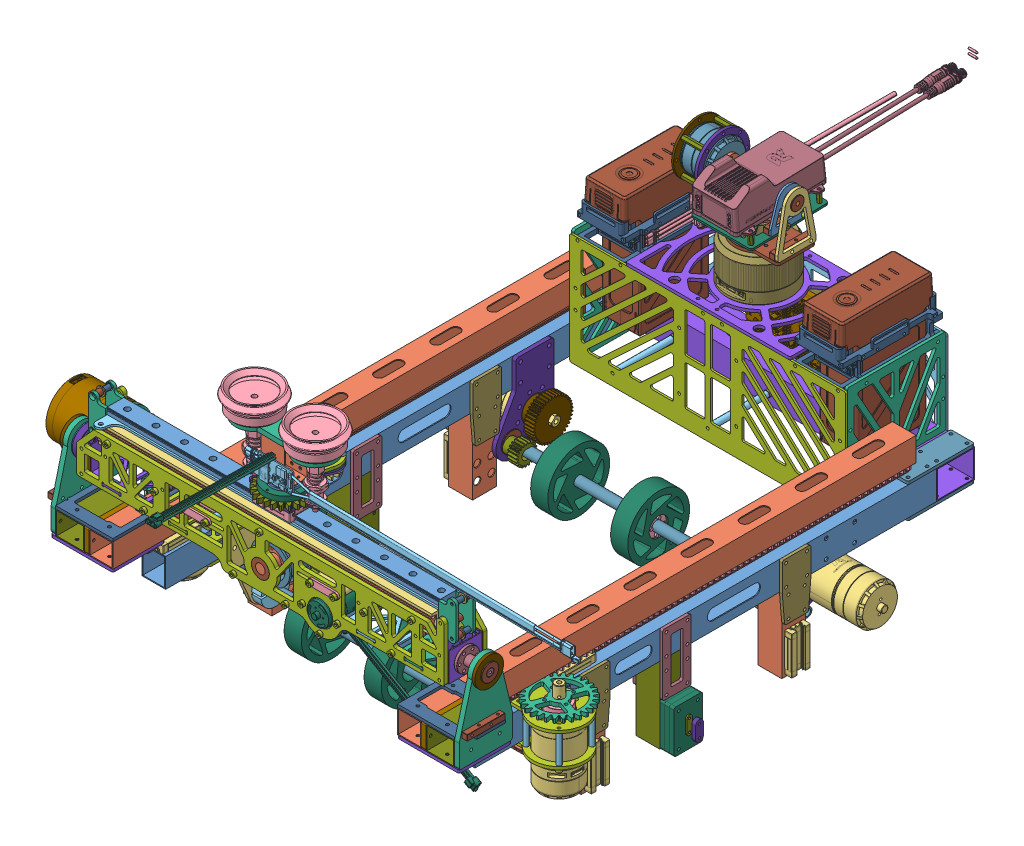
SolidWorks assembly 上层框架总装1.0, configuration 默认. Lengths in mm. (continued)
Components (placement in the parent): (continued)
- 取矿横移总装-1: 取矿横移总装 [默认] at (0 138 270.5) x (0 0 -1) z (1 0 0) size (203.34 276.76 526.28) (continued)
  - 横移总装2.0-1: 横移总装2.0 [默认] at origin size (67.7 199.63 415.26) (continued)
    - 12.9级圆柱头螺钉-15: 12.9级圆柱头螺钉 [M3*10] at (-27.5 -18 -80) x (0 -0.999995 -0.003259) z (-1 0 0) size (5.68 5.68 13)
    - 12.9级圆柱头螺钉-16: 12.9级圆柱头螺钉 [M3*10] at (-27.5 -18 -55) x (0 -0.999995 -0.003259) z (-1 0 0) size (5.68 5.68 13)
    - 12.9级圆柱头螺钉-17: 12.9级圆柱头螺钉 [M3*10] at (-25.5 -52 -27.5) x (0 -0.999995 -0.003259) z (-1 0 0) size (5.68 5.68 13)
    - 12.9级圆柱头螺钉-18: 12.9级圆柱头螺钉 [M3*10] at (-25.5 -52 27.5) x (0 -0.999995 -0.003259) z (-1 0 0) size (5.68 5.68 13)
    - 12.9级圆柱头螺钉-19: 12.9级圆柱头螺钉 [M3*10] at (-25.5 -42.8 44.6275) x (0 -0.999995 -0.003259) z (-1 0 0) size (5.68 5.68 13)
    - 12.9级圆柱头螺钉-20: 12.9级圆柱头螺钉 [M3*10] at (-27.5 -18 55) x (0 -0.999995 -0.003259) z (-1 0 0) size (5.68 5.68 13)
    - 12.9级圆柱头螺钉-21: 12.9级圆柱头螺钉 [M3*10] at (-27.5 -18 80) x (0 -0.999995 -0.003259) z (-1 0 0) size (5.68 5.68 13)
    - 12.9级圆柱头螺钉-22: 12.9级圆柱头螺钉 [M3*10] at (-25.5 -61.3122 63.1397) x (0 -0.999995 -0.003259) z (-1 0 0) size (5.68 5.68 13)
    - 12.9级圆柱头螺钉-23: 12.9级圆柱头螺钉 [M3*10] at (-25.5 -42.8 81.6519) x (0 -0.999995 -0.003259) z (-1 0 0) size (5.68 5.68 13)
    - 12.9级圆柱头螺钉-24: 12.9级圆柱头螺钉 [M3*10] at (-25.5 -18 110) x (0 -0.999995 -0.003259) z (-1 0 0) size (5.68 5.68 13)
    - 12.9级圆柱头螺钉-25: 12.9级圆柱头螺钉 [M3*10] at (-25.5 -41 138.7695) x (0 -0.999995 -0.003259) z (-1 0 0) size (5.68 5.68 13)
    - 12.9级圆柱头螺钉-26: 12.9级圆柱头螺钉 [M3*8] at (-25.5 0 160) x (0 -0.999995 -0.003259) z (-1 0 0) size (5.68 5.68 11)
    - 12.9级圆柱头螺钉-27: 12.9级圆柱头螺钉 [M3*8] at (-25.5 0 0) x (0 -0.999995 -0.003259) z (-1 0 0) size (5.68 5.68 11)
    - 12.9级圆柱头螺钉-28: 12.9级圆柱头螺钉 [M3*8] at (-25.5 0 -160) x (0 -0.999995 -0.003259) z (-1 0 0) size (5.68 5.68 11)
    - 12.9级圆柱头螺钉-29: 12.9级圆柱头螺钉 [M3*8] at (25.5 0 -160) x (0 -0.774925 -0.632053) z (1 0 0) size (5.68 5.68 11)
    - 12.9级圆柱头螺钉-30: 12.9级圆柱头螺钉 [M3*8] at (25.5 0 0) x (0 -0.774925 -0.632053) z (1 0 0) size (5.68 5.68 11)
    - 12.9级圆柱头螺钉-31: 12.9级圆柱头螺钉 [M3*8] at (25.5 0 160) x (0 -0.774925 -0.632053) z (1 0 0) size (5.68 5.68 11)
    - 304不锈钢平头倒边螺丝-1: 304不锈钢平头倒边螺丝 [M3*10] at (24.3 -52 27.5) x (0 0.904522 -0.426427) z (1 0 0) size (7 7 11.8)
    - 12.9级圆柱头螺钉-32: 12.9级圆柱头螺钉 [M3*10] at (25.5 -42.8 44.6275) x (0 -0.265301 -0.964166) z (1 0 0) size (5.68 5.68 13)
    - 转点法兰-1: 转点法兰 [默认] at (0 -30 193) x (0.866025 0.5 0) z (0 0 1) size (24 24 26)
  - 吸盘总装-1: 吸盘总装 [默认] at (0 34 3.3555) x (-1 0 0) z (0 1 0) size (203.34 428.51 86.1)
    - 6750zz-1: 6750zz [默认] at origin size (32 32 4)
    - 轴承外圈固定-1: 轴承外圈固定 [默认] at (0 0 0.03) x (0 -1 0) z (0 0 1) size (42 42 5.34)
    - 圆柱齿轮24×2-1: 圆柱齿轮24×2 [默认] at (0 0 -4.5) size (51.72 51.72 5)
    - 拉线安装版-1: 拉线安装版 [默认] at (0 0 -10) x (0 1 0) z (0 0 1) size (63.3 30 3)
    - 内圈分离铝件-1: 内圈分离铝件 [默认] at (0 0 1.95) x (-0.717753 -0.696298 0) z (0 0 -1) size (28 28 5.15)
    - 内圈压板-1: 内圈压板 [默认] at (0 0 2) x (0.717753 0.696298 0) z (0 0 1) size (28 28 3)
    - 20x40x1铝方管-2: 20x40x1铝方管 [默认] at (0 0 25) x (-0.999885 0.015171 0) z (0.015171 0.999885 0) size (25 40 25)
    - RoboMaster M2006 P36直流无刷减速电机-1: RoboMaster M2006 P36直流无刷减速电机 [默认] at (-58.4085 2.0306 32.7952) x (-0.717753 -0.696298 0) z (0 0 1) size (140.17 141.41 64.8)
    - 圆柱齿轮14×2-1: 圆柱齿轮14×2 [默认] at (-37.9956 0.5765 -4.5) x (-0.882361 0.470573 0) z (0 0 1) size (32 31.46 3)
    - 推力球轴承-1: 推力球轴承 [F6-12M 6*12*4] at (-37.9956 0.5765 -3) x (0.191226 -0.981546 0) z (-0.981546 -0.191226 0) size (12 4 12)
    - 吸盘-1: 吸盘 [PJTS-50-6-N] at (-0.493 -32.4963 72) x (-0.999885 0.015171 0) z (-0.015171 -0.999885 0) size (54.83 80 54.83)
    - 吸盘-2: 吸盘 [PJTS-50-6-N] at (0.493 32.4963 72) x (0.996645 0.081841 0) z (-0.081841 0.996645 0) size (54.83 80 54.83)
    - C610无刷电机调速器-1: C610无刷电机调速器 [默认] at (16.0987 6.3023 -120.7197) x (0 0 -1) z (0.999885 -0.015171 0) size (22.14 353.32 7.25)
    - 吸盘固定板2-1: 吸盘固定板2 [默认] at (0 0 45) x (0.015171 0.999885 0) z (0 0 1) size (105 40 5)
    - 2006电机紧固板-1: 2006电机紧固板 [默认] at (-37.9956 0.5765 8) x (0.999885 -0.015171 0) z (0 0 -1) size (43.75 36.5 3)
    - 2006电机安装板-1: 2006电机安装板 [默认] at (-37.9956 0.5765 0.9) x (-0.999885 0.015171 0) z (0 0 1) size (35.09 36.5 2)
    - 2006电机紧固板-2: 2006电机紧固板 [默认] at (-37.9956 0.5765 29) x (0.999885 -0.015171 0) z (0 0 -1) size (43.75 36.5 3)
    - 304不锈钢接线柱-1: 304不锈钢接线柱 [M3*18-6] at (-48.9414 -10.0421 17) size (6 6 18)
    - 304不锈钢接线柱-2: 304不锈钢接线柱 [M3*18-6] at (-48.6142 11.5222 17) x (-0.15981 -0.987148 0) z (0 0 1) size (6 6 18)
    - 304不锈钢接线柱-3: 304不锈钢接线柱 [M3*18-6] at (-27.0499 11.195 17) size (6 6 18)
    - 304不锈钢接线柱-4: 304不锈钢接线柱 [M3*18-6] at (-27.3771 -10.3692 17) size (6 6 18)
    - 安装铝件-1: 安装铝件 [默认] at (-15.4982 0.2351 17) x (-0.015171 -0.999885 0) z (0.999885 -0.015171 0) size (25 18 6)
    - 2006电机安装垫块-1: 2006电机安装垫块 [默认] at (-37.9956 0.5765 3.95) x (-0.999885 0.015171 0) z (0 0 1) size (35.09 36.5 2.1)
- 金矿石-1: 金矿石 [默认] at (1548.9384 -999.1063 260.5454) size (200 200 200) (hidden)
- 器件模块总装1.0-1: 器件模块总装1.0 [默认] at (0 150 -230.75) size (300.9 248.89 343.45)
  - 图传云台模块-1: 图传云台模块 [默认] at origin size (115.96 130.39 343.45) (flexible)
    - 6020电机传动板-1: 6020电机传动板 [默认] x (1 0 0) z (0 -1 0) size (80 50 3)
    - RoboMaster GM6020 直流无刷电机-1: RoboMaster GM6020 直流无刷电机 [默认] at (0 72.0479 0) x (-0.5 0 -0.866025) z (0 1 0) size (66.7 66.7 45)
    - RoboMaster 图传模块 VT02 2019-1: RoboMaster 图传模块 VT02 2019 [默认] at (0 34.005 -0.333) x (-1 0 0) z (0 0.03027 -0.999542) size (60 36.29 258.03)
    - RoboMaster M3508直流无刷电机转子-1: RoboMaster M3508直流无刷电机转子 [默认] at (-11.659 32.3995 -13.3475) x (0 -0.790596 0.612338) z (-1 0 0) size (42 42 43.4)
    - 图传安装板-1: 图传安装板 [默认] at (0 20.0115 -0.7568) x (1 0 0) z (0 -0.999542 -0.03027) size (64 82 2)
    - 304不锈钢柱-1: 304不锈钢柱 [M2*10] at (27 23.9194 35.3781) x (-0.601616 -0.02418 0.798419) z (0 -0.999542 -0.03027) size (4.62 4 10)
    - 304不锈钢柱-2: 304不锈钢柱 [M2*10] at (-27 23.9194 35.3781) x (-0.601616 -0.02418 0.798419) z (0 -0.999542 -0.03027) size (4.62 4 10)
    - 304不锈钢柱-3: 304不锈钢柱 [M2*10] at (27 26.0989 -36.5889) x (-0.956324 -0.008848 0.292175) z (0 -0.999542 -0.03027) size (4.62 4 10)
    - 304不锈钢柱-4: 304不锈钢柱 [M2*10] at (-27 26.0989 -36.5889) x (0.570383 -0.024864 0.821002) z (0 -0.999542 -0.03027) size (4.62 4 10)
    - 四孔直角转接件-1: 四孔直角转接件 [上交角件] at (-26 23.0101 -0.666) x (1 0 0) z (0 -0.03027 0.999542) size (6 6 40)
    - 四孔直角转接件-2: 四孔直角转接件 [上交角件] at (27 23.0101 -0.666) x (1 0 0) z (0 -0.03027 0.999542) size (6 6 40)
    - 云台转接板-1: 云台转接板 [默认] at (-37 45 0) x (0 0 1) z (-1 0 0) size (55 72.5 3.26)
    - 3508定子安装板-1: 3508定子安装板 [默认] at (-64.1 45 0) x (0 0.707107 -0.707107) z (1 0 0) size (55 55 2)
    - 云台旋转板-1: 云台旋转板 [默认] at (32 45 0) x (0 -0.03027 0.999542) z (-1 0 0) size (40 37.5 2)
    - 3508传动板-1: 3508传动板 [默认] at (-32 45 0) x (0 0.03027 -0.999542) z (1 0 0) size (40 34.5 3)
    - 法兰轴承-1: 法兰轴承 [4*12*4-1] at (41 45 0) x (0 0.036514 0.999333) z (0 -0.999333 0.036514) size (13.5 4 13.5)
    - 转接板2-1: 转接板2 [默认] at (37 45 0) x (0 0 -1) z (1 0 0) size (40 57.5 3)
    - 推力球轴承-1: 推力球轴承 [F4-9M 4*9*4] at (37 45 0) x (0 0.757396 -0.652956) z (0 0.652956 0.757396) size (9 4 9)
    - 法兰轴承-2: 法兰轴承 [4*12*4-1] at (29 45 0) x (0 -0.234612 -0.972089) z (0 -0.972089 0.234612) size (13.5 4 13.5)
    - 304不锈钢柱-5: 304不锈钢柱 [M3*22] at (-51 27.6759 17.3241) x (0 -0.514688 -0.857378) z (1 0 0) size (5.43 4.7 22)
    - 304不锈钢柱-6: 304不锈钢柱 [M3*22] at (-51 27.6759 -17.3241) x (0 -0.372237 -0.928138) z (1 0 0) size (5.43 4.7 22)
    - 304不锈钢柱-7: 304不锈钢柱 [M3*22] at (-51 62.3241 -17.3241) x (0 -0.251026 -0.96798) z (1 0 0) size (5.43 4.7 22)
    - 304不锈钢柱-8: 304不锈钢柱 [M3*22] at (-51 62.3241 17.3241) x (0 -0.159705 -0.987165) z (1 0 0) size (5.43 4.7 22)
    - 四孔直角转接件-3: 四孔直角转接件 [上交角件] at (34 3 0) size (6 6 40)
    - 四孔直角转接件-4: 四孔直角转接件 [上交角件] at (-34 3 0) size (6 6 40)
    - C620无刷电机调速器-1: C620无刷电机调速器 [默认] at (-45.4 6.2704 2.5313) x (0 0 1) z (0 1 0) size (343.45 13.81 26.13)
    - 12.9级圆柱头螺钉-1: 12.9级圆柱头螺钉 [M3*8] at (35 22.8587 4.3318) x (0 -0.455873 -0.890045) z (1 0 0) size (5.68 5.68 11)
    - 12.9级圆柱头螺钉-2: 12.9级圆柱头螺钉 [M3*8] at (35 23.4641 -15.6591) x (0 -0.455873 -0.890045) z (1 0 0) size (5.68 5.68 11)
  - 上层器件安装背板-1: 上层器件安装背板 [默认] at (0 -106.5 -52.75) size (290 117 2)
  - 元器件安装侧板-1: 元器件安装侧板 [默认] at (143.5 -90 0) x (0 0 -1) z (1 0 0) size (103.5 120 3)
  - 元器件安装侧板-2: 元器件安装侧板 [默认] at (-143.5 -90 0) x (0 0 -1) z (1 0 0) size (103.5 120 3)
  - 元器件安装前板-1: 元器件安装前板 [默认] at (0 -106.5 52.75) size (290 117 2)
  - 元器件安装上板-1: 元器件安装上板 [默认] at (0 -46.5 0) x (-1 0 0) z (0 1 0) size (173 107.5 3)
  - 开发板A型-1: 开发板A型 [默认] at (-195.9 -96.5 -343.1489) x (0 -1 0) z (0 0 -1) size (58.4 85.42 16.4)
  - 电池装配体-1: 电池装配体 [默认] at (-17.7524 -28.2099 12.1891) x (0 0 1) z (-1 0 0) size (103.5 134.81 69.3)
    - RoboMaster 电池架（兼容型）-1: RoboMaster 电池架（兼容型） [Default] at (-57.9391 2.2099 96.5476) size (103.5 37.5 69.3)
    - TB47S电池-1: TB47S电池 [默认] at (-59.0391 2.7599 97.3476) size (101.5 134.81 44.3)
  - 电池装配体-2: 电池装配体 [默认] at (210.8476 -28.2099 12.1891) x (0 0 1) z (-1 0 0) size (103.5 134.81 69.3)
    - RoboMaster 电池架（兼容型）-1: RoboMaster 电池架（兼容型） [Default] at (-57.9391 2.2099 96.5476) size (103.5 37.5 69.3)
    - TB47S电池-1: TB47S电池 [默认] at (-59.0391 2.7599 97.3476) size (101.5 134.81 44.3)
  - 四孔直角转接件-1: 四孔直角转接件 [上交角件] at (-139 -100 48.75) x (1 0 0) z (0 -1 0) size (6 6 40)
  - 四孔直角转接件-2: 四孔直角转接件 [上交角件] at (-139 -100 -48.75) x (1 0 0) z (0 -1 0) size (6 6 40)
  - 四孔直角转接件-3: 四孔直角转接件 [上交角件] at (0 -51 48.75) x (0 1 0) z (1 0 0) size (6 6 40)
  - a板安装板-1: a板安装板 [默认] at (0 -97 -41.75) x (0 -1 0) z (-1 0 0) size (72 2 99)
  - 304不锈钢接线柱-1: 304不锈钢接线柱 [M3*10-6] at (-46.5 -130 -46.75) size (6 6 10)
  - 304不锈钢接线柱-2: 304不锈钢接线柱 [M3*10-6] at (-46.5 -64 -46.75) x (0.999692 0.02482 0) z (0 0 1) size (6 6 10)
  - 304不锈钢接线柱-3: 304不锈钢接线柱 [M3*10-6] at (46.5 -130 -46.75) x (0.988734 0.149683 0) z (0 0 1) size (6 6 10)
  - 304不锈钢接线柱-4: 304不锈钢接线柱 [M3*10-6] at (46.5 -64 -46.75) x (0.988734 0.149683 0) z (0 0 1) size (6 6 10)
- 304不锈钢接线柱-1: 304不锈钢接线柱 [M3*60-6] at (100 -3 -209) x (0.581063 -0.813858 0) z (0 0 1) size (6 6 60)
- 打印件垫块-1: 打印件垫块 [默认] at (100 -3 -242.5) size (6.5 6.5 3.5)
- 304不锈钢接线柱-2: 304不锈钢接线柱 [M3*60-6] at (0 -3 -209) x (0.523113 0.852263 0) z (0 0 1) size (6 6 60)
- 304不锈钢接线柱-3: 304不锈钢接线柱 [M3*60-6] at (-100 -3 -209) x (0.523113 0.852263 0) z (0 0 1) size (6 6 60)
- 打印件垫块-2: 打印件垫块 [默认] at (0 -3 -242.5) size (6.5 6.5 3.5)
- 打印件垫块-3: 打印件垫块 [默认] at (-100 -3 -242.5) x (0.999701 0.024449 0) z (0 0 1) size (6.5 6.5 3.5)
- 前后翻矿机构-1: 前后翻矿机构 [默认] at (0 -58 13) x (0 0 1) z (-1 0 0) size (360.93 118.11 442.2)
  - 10mm铝管-1: 10mm铝管 [默认] at (-129.5 0 0) x (1 0 0) z (0 0 -1) size (10 10 330)
  - 10mm铝管-2: 10mm铝管 [默认] at (129.5 0 0) x (-1 0 0) z (0 0 -1) size (10 10 330)
  - 翻矿打印件-1: 翻矿打印件 [默认] at (129.5 0 84) x (0.829736 0.558156 0) z (0 0 1) size (65 65 18)
  - 翻矿打印件-2: 翻矿打印件 [默认] at (129.5 0 -84) x (0.990398 0.138246 0) z (0 0 1) size (65 65 18)
  - 翻矿打印件-3: 翻矿打印件 [默认] at (-129.5 0 -84) x (-0.047381 0.998877 0) z (0 0 1) size (65 65 18)
  - 翻矿打印件-4: 翻矿打印件 [默认] at (-129.5 0 84) x (0.911199 0.411966 0) z (0 0 1) size (65 65 18)
  - 圆柱齿轮20×1-1: 圆柱齿轮20×1 [默认] at (-125.8171 0 126) x (-0.64056 -0.767908 0) z (0 0 1) size (21.83 21.83 18)
  - 法兰轴承-1: 法兰轴承 [10*19*5-1] at (-129.5 0 145) x (0.582685 0.812698 0) z (0.812698 -0.582685 0) size (21 5 21)
  - 翻矿电机安装板-2: 翻矿电机安装板 [后驱] at (-129.5 0 150) x (-1 0 0) z (0 0 -1) size (61 89 4)
  - RoboMaster M3508直流无刷减速电机-1: RoboMaster M3508直流无刷减速电机 [默认] at (-162.6696 2.0988 236.441) x (-0.91084 0.412759 0) z (0 0 -1) size (42 42.01 98.4)
  - 圆柱齿轮40×1-1: 圆柱齿轮40×1 [默认] at (-153.5 18 126) x (0.992313 -0.123751 0) z (0 0 1) size (41.92 41.92 20)
  - 翻矿电机安装板-3: 翻矿电机安装板 [前驱] at (-129.5 0 -146) x (-1 0 0) z (0 0 -1) size (62.48 89 4)
  - RoboMaster M3508直流无刷减速电机-2: RoboMaster M3508直流无刷减速电机 [默认] at (-161.5702 0.8682 -236.441) x (0.893896 -0.448274 0) z (0 0 1) size (42 42.01 98.4)
  - 法兰轴承-2: 法兰轴承 [10*19*5-1] at (-129.5 0 -145) x (-0.831063 -0.556179 0) z (0.556179 -0.831063 0) size (21 5 21)
  - 大带轮5mx29-1: 大带轮5mx29 [A] at (-154.98 18 -72.58) x (0 0 -1) z (0.816888 -0.576796 0) size (10 44.91 44.97)
  - 小带轮5mx18-1: 小带轮5mx18 [默认] at (129.5 0 -121) x (0 0 -1) z (0.777037 -0.629455 0) size (21 27.19 27.51)
  - 推力球轴承-1: 推力球轴承 [51100 10*24*9] at (-154.98 18 -148.08) x (-0.468033 -0.883711 0) z (-0.883711 0.468033 0) size (24 9 24)
  - 翻矿前连接板-1: 翻矿前连接板 [默认] at (129.5 0 -150) size (53 89.5 4)
  - 法兰轴承-3: 法兰轴承 [10*19*5-1] at (129.5 0 -145) x (-0.896596 -0.442849 0) z (0.442849 -0.896596 0) size (21 5 21)
  - 翻矿前连接板-2: 翻矿前连接板 [默认] at (129.5 0 146) size (53 89.5 4)
  - 法兰轴承-4: 法兰轴承 [10*19*5-1] at (129.5 0 145) x (0.110634 -0.993861 0) z (-0.993861 -0.110634 0) size (21 5 21)
  - Z21-10-20-13-1: Z21-10-20-13 [默认] at (129.5 0 84.5) size (20 20 15)
  - Z21-10-20-13-2: Z21-10-20-13 [默认] at (129.5 0 -83.5) x (0.99719 0.074916 0) z (0 0 1) size (20 20 15)
  - Z21-10-20-13-3: Z21-10-20-13 [默认] at (-129.5 0 -83.5) x (0.999856 0.016974 0) z (0 0 1) size (20 20 15)
  - Z21-10-20-13-4: Z21-10-20-13 [默认] at (-129.5 0 84.5) x (0.884281 0.466955 0) z (0 0 1) size (20 20 15)
  - 翻矿打印件-5: 翻矿打印件 [默认] at (129.5 0 0) x (-0.967813 -0.251669 0) z (0 0 -1) size (65 65 18)
  - 翻矿打印件-6: 翻矿打印件 [默认] at (-129.5 0 0) x (-0.931626 -0.363419 0) z (0 0 -1) size (65 65 18)
  - Z21-10-20-13-5: Z21-10-20-13 [默认] at (-129.5 0 -0.5) x (-0.987188 -0.159561 0) z (0 0 -1) size (20 20 15)
  - 紧固环-1: 紧固环 [默认] at (129.5 0 139.7) size (29.93 30 10)
  - 限位打印件-1: 限位打印件 [默认] at (-129.5 0 -119) size (14 14 52)
Mates (geometry in assembly coordinates):
- 重合2: coincident aligned: plane of 取矿横移总装-1/横移总装2.0-1 through (0 138 270.5) normal (1 0 0)
- 平行3: parallel anti-aligned: plane of 前探2.0-1/25x25x1铝方管-2 through (150 53 303.4607) normal (0 1 0); plane of 取矿横移总装-1/横移总装2.0-1/安装固定板-2 through (0 118 297.4607) normal (0 0 1)
- 平行4: parallel aligned: plane of 前探2.0-1/25x25x1铝方管-2 through (162.5 40.5 303.4607) normal (0 0 1); plane of 取矿横移总装-1/横移总装2.0-1/安装固定板-2 through (0 118 297.4607) normal (0 0 1)
- 重合6: coincident aligned: plane of 器件模块总装1.0-1 through (0 150 -230.75) normal (1 0 0)
- 重合7: coincident anti-aligned: plane of 前探2.0-1/30x40x1铝方管-4 through (190 15 -242.5) normal (0 1 0); plane of 器件模块总装1.0-1/元器件安装侧板-1 through (145 15 -179) normal (0 -1 0)
- 重合8: coincident anti-aligned: plane of 前探2.0-1/30x40x1铝方管-4 through (190 -15 -282.5) normal (0 0 -1); plane of 器件模块总装1.0-1/上层器件安装背板-1 through (0 43.5 -282.5) normal (0 0 1)
- 重合9: coincident anti-aligned: plane of 前探2.0-1/30x40x1铝方管-4 through (190 15 -242.5) normal (0 1 0); plane of 器件模块总装1.0-1/开发板A型-1 through (0 53 -270.5) normal (0 0 -1)
- 同心4: concentric aligned: cylinder of 取矿横移总装-1/横移总装2.0-1/35x10x1铝方管-1 through (183 108 270.5) axis (1 0 0) radius 4; cylinder of 前探2.0-1/横移连接板-2 through (201 108 270.5) axis (1 0 0) radius 8
- 平行5: parallel aligned: plane of 前探2.0-1/横移连接板-2 through (123.1167 31 299) normal (0 0 1); plane of 取矿横移总装-1/横移总装2.0-1/安装固定板-2 through (0 118 293) normal (0 0 1)
- 重合10: coincident anti-aligned: plane of 前探2.0-1/40x30x1铝方管-1 through (-175 -15 -282.5) normal (0 0 -1); plane of 器件模块总装1.0-1/上层器件安装背板-1 through (0 43.5 -282.5) normal (0 0 1)
- 重合11: coincident anti-aligned: plane of 前探2.0-1/40x30x1铝方管-1 through (-175 15 -282.5) normal (0 1 0); plane of 器件模块总装1.0-1/元器件安装侧板-2 through (-142 15 -179) normal (0 -1 0)
- 重合12: coincident anti-aligned: plane of 器件模块总装1.0-1/元器件安装前板-1 through (0 43.5 -179) normal (0 0 -1); plane of 304不锈钢接线柱-1 through (102.4416 -1.2568 -179) normal (0 0 1)
- 同心5: concentric anti-aligned: cylinder of 304不锈钢接线柱-1 through (100 -3 -179) axis (0 0 1) radius 3; cylinder of 打印件垫块-1 through (100 -3 -239) axis (0 0 -1) radius 3.25
- 重合13: coincident anti-aligned: plane of 前探2.0-1/40x30x1铝方管-1 through (-175 -15 -242.5) normal (0 0 1); plane of 打印件垫块-1 through (100 -3 -242.5) normal (0 0 -1)
- 同心6: concentric aligned: cylinder of 器件模块总装1.0-1/元器件安装前板-1 through (100 -3 -187) axis (0 0 1) radius 1.525; cylinder of 304不锈钢接线柱-1 through (100 -3 -179) axis (0 0 1) radius 3
- 同心7: concentric aligned: cylinder of 器件模块总装1.0-1/元器件安装前板-1 through (0 -3 -187) axis (0 0 1) radius 1.525; cylinder of 304不锈钢接线柱-2 through (0 -3 -179) axis (0 0 1) radius 3
- 重合14: coincident anti-aligned: plane of 器件模块总装1.0-1/元器件安装前板-1 through (0 43.5 -179) normal (0 0 -1); plane of 304不锈钢接线柱-2 through (-2.5568 -1.4307 -179) normal (0 0 1)
- 同心8: concentric anti-aligned: circle of 器件模块总装1.0-1/元器件安装前板-1; cylinder of 304不锈钢接线柱-3 through (-100 -3 -179) axis (0 0 1) radius 3
- 重合15: coincident anti-aligned: plane of 器件模块总装1.0-1/元器件安装前板-1 through (0 43.5 -179) normal (0 0 -1); plane of 304不锈钢接线柱-3 through (-102.5568 -1.4307 -179) normal (0 0 1)
- 重合16: coincident anti-aligned: plane of 304不锈钢接线柱-2 through (0 -3 -239) normal (0 0 -1); plane of 打印件垫块-2 through (0 -3 -239) normal (0 0 1)
- 同心9: concentric anti-aligned: cylinder of 304不锈钢接线柱-2 through (0 -3 -179) axis (0 0 1) radius 3; cylinder of 打印件垫块-2 through (0 -3 -239) axis (0 0 -1) radius 3.25
- 同心10: concentric anti-aligned: cylinder of 304不锈钢接线柱-3 through (-100 -3 -179) axis (0 0 1) radius 3; cylinder of 打印件垫块-3 through (-100 -3 -239) axis (0 0 -1) radius 3.25
- 重合17: coincident anti-aligned: plane of 304不锈钢接线柱-3 through (-100 -3 -239) normal (0 0 -1); plane of 打印件垫块-3 through (-100 -3 -239) normal (0 0 1)
- 平行6: parallel aligned: plane of 前探2.0-1/25x25x1铝方管-2 through (150 56 299) normal (0 1 0); plane of 前后翻矿机构-1 through (0 -58 13) normal (0 1 0)
- 重合18: coincident anti-aligned: plane of 前后翻矿机构-1 through (0 -58 13) normal (-1 0 0)
- 对称1: symmetric aligned: plane of 前探2.0-1/25x25x1铝方管-3 through (150 -95 105.9) normal (0 0 -1); plane of 前后翻矿机构-1 through (150 -95 -79.9) normal (0 0 1); plane of 前探2.0-1/25x25x1铝方管-4 through (0 -58 13) normal (0 0 1)
- 距离1: distance = 43 mm: cylinder of 前后翻矿机构-1/10mm铝管-2 through (165 -58 142.5) axis (-1 0 0) radius 5; plane of 前探2.0-1/30x25x1铝方管-2 through (150 -15 242.5) normal (0 -1 0)
